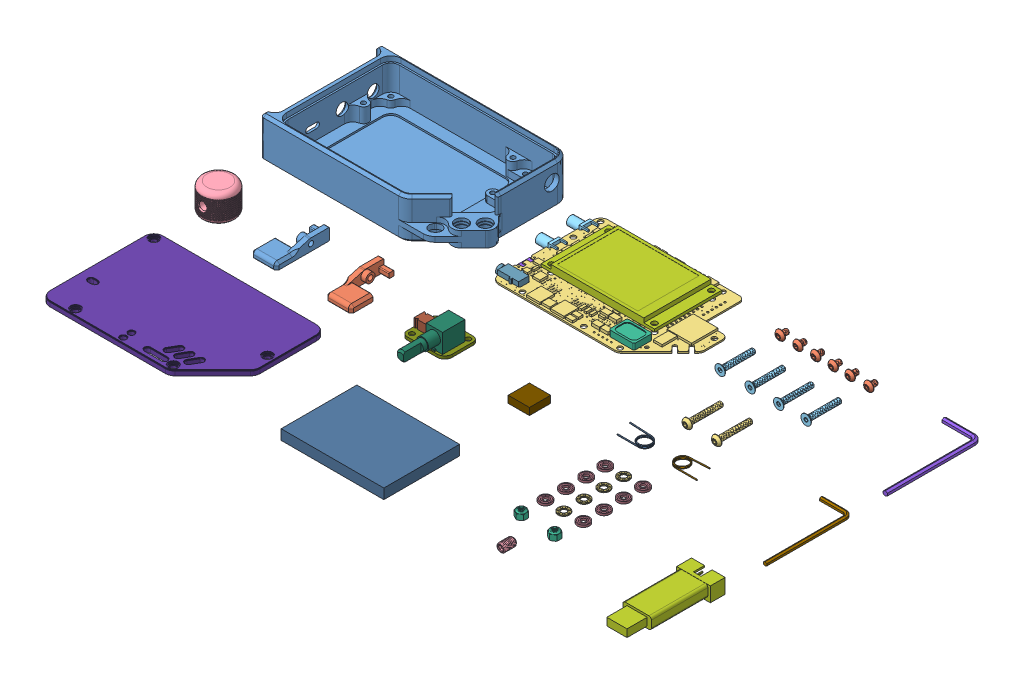
SolidWorks assembly PSDR Parts, configuration Default. Lengths in mm.
Overall size (359.88 28.12 210.13).
49 component instances, 28 part files, 92 mates.
Components (placement in the parent):
- BottomHalf2-1: BottomHalf2 [Default] at (9 12.38 68.5) x (1 0 0) z (0 1 0) size (118.23 72 24.11)
- 92095A471_18-8 SS BUTTON-HEAD SOCKET CAP SCREW-1: 92095A471_18-8 SS BUTTON-HEAD SOCKET CAP SCREW [92095A471] at (297.198 0 9.1982) x (-0.787462 -0.616364 0) z (0 0 1) size (5.7 5.7 5.93)
- 92095A185_18-8 SS BUTTON-HEAD SOCKET CAP SCREW-1: 92095A185_18-8 SS BUTTON-HEAD SOCKET CAP SCREW [92095A185] at (279.901 0 82.2808) x (0.394049 -0.919089 0) z (0 0 1) size (5.7 5.7 22.02)
- 92095A471_18-8 SS BUTTON-HEAD SOCKET CAP SCREW-2: 92095A471_18-8 SS BUTTON-HEAD SOCKET CAP SCREW [92095A471] at (244.5337 0 9.1982) x (0.999368 0.035541 0) z (0 0 1) size (5.7 5.7 5.93)
- 92029A208_TYPE 316 STAINLESS STEEL CUP POINT SET SCREW-1: 92029A208_TYPE 316 STAINLESS STEEL CUP POINT SET SCREW [92029A208] at (271.0951 0 196.8779) x (0.086276 0.996271 0) z (0 0 1) size (5.17 5.13 8.8)
- 93395A213_TYPE 316 SS FLAT-HEAD SOCKET CAP SCREW-1: 93395A213_TYPE 316 SS FLAT-HEAD SOCKET CAP SCREW [93395A213] at (244.6789 0 43.7019) x (-0.136325 -0.990664 0) z (0 0 1) size (6 6 20.36)
- 94205A220_TYPE 316 STAINLESS STEEL NYLON-INSERT LOCKNUT-1: 94205A220_TYPE 316 STAINLESS STEEL NYLON-INSERT LOCKNUT [94205A220] at (261.1628 0 178.1232) size (5.5 4.1 6.35)
- 2.2in_LCD_Module-1: 2.2in_LCD_Module [Default] at (178.3977 6.3051 29.9486) x (-1 0 0) z (0 0 -1) size (67.3 4.15 40)
- 2.5mm_Allen_Wrench-1: 2.5mm_Allen_Wrench [Default] at (357.3787 0.7217 59.475) x (0 0 1) z (-1 0 0) size (56.47 2.89 21.55)
- 2mm_Allen_Wrench-1: 2mm_Allen_Wrench [Default] at (357.8787 0.5774 131.1017) x (0 0 1) z (-1 0 0) size (51.21 2.31 17.88)
- 604561 Battery-1: 604561 Battery [Default] at (180.9722 0 187.6347) size (61 6 45)
- Battery Connector-1: Battery Connector [Default] at (139.5256 1.68 111.229) x (0 0 -1) z (1 0 0) size (6 8.6 10)
- Bearing_Inside-1: Bearing_Inside [Default] at (271.1658 0.3 162.9376) x (-0.834175 0 -0.5515) z (0.5515 0 -0.834175) size (6.7 1.25 6.7)
- Bearing_Outside-1: Bearing_Outside [Default] at (282.6637 0 150.5673) size (7 1.25 7)
- Earphone_Jack-1: Earphone_Jack [Default] at (133.0998 6.1 61.0044) x (1 0 0) z (0 0 -1) size (14.3 5.7 8.4)
- Encoder-1: Encoder [Default] at (155.9304 1.68 106.4098) x (0 0 1) z (-1 0 0) size (33.3 11.35 9.7)
- EncoderBoard-1: EncoderBoard [Default] at (93.5977 4.7 21.1162) x (0 0 1) z (0 1 0) size (20 25.5 1.68)
- Face Cover4-1: Face Cover4 [Default] at (8.7 -8.62 208.9347) x (1 0 0) z (0 1 0) size (102.4 67.4 3)
- Foam_Square-1: Foam_Square [Default] at (205.1722 0 117.3729) size (12.6 4.2 12.6)
- paddle-1: paddle [Default] at (56.1722 4 104.0749) x (0 0 1) z (0 1 0) size (31.7 15.5 7)
- paddle_Mirrored-1: paddle_Mirrored [Default] at (97.4502 4 104.0749) x (0 0 1) z (0 -1 0) size (31.7 15.5 7)
- PSDR26PCB-1: PSDR26PCB [Default] at (133.0977 2.5 67.9986) x (1 0 0) z (0 1 0) size (100 65 5.1)
- Slotted_Knob2-1: Slotted_Knob2 [Default] at (14.2624 0 111.1139) size (20.37 16 20.31)
- SMA_Connector-1: SMA_Connector [Default] at (135.0535 2.125 31.5236) x (1 0 0) z (0 0 -1) size (13.33 6.35 6.35)
- Speaker-1: Speaker [Default] at (205.0112 3.3992 57.0766) size (15 3.5 11)
- ST-Link-1: ST-Link [Default] at (349.8787 3.5 210.1347) size (20 8.7 54.3)
- USB_Connector-1: USB_Connector [Default] at (133.9105 2.5 49.0064) x (0 0 -1) z (-1 0 0) size (8.2 3.33 4.94)
- SMA_Connector-2: SMA_Connector [Default] at (135.0535 2.125 13.0361) x (1 0 0) z (0 0 -1) size (13.33 6.35 6.35)
- LeeSpring-LTML060L08S-1: LeeSpring-LTML060L08S [Default] at (282.1263 0.3047 103.5123) x (0.999674 0.025542 0) z (0 0 1) size (17.33 2.81 8.24)
- LeeSpring-LTMR060L08S-1: LeeSpring-LTMR060L08S [Default] at (260.0829 0.3047 103.7248) x (0.999674 -0.025542 0) z (0 0 1) size (17.33 2.81 8.24)
- 92095A471_18-8 SS BUTTON-HEAD SOCKET CAP SCREW-3: 92095A471_18-8 SS BUTTON-HEAD SOCKET CAP SCREW [92095A471] at (276.0216 0 9.1982) size (5.7 5.7 5.93)
- 92095A471_18-8 SS BUTTON-HEAD SOCKET CAP SCREW-4: 92095A471_18-8 SS BUTTON-HEAD SOCKET CAP SCREW [92095A471] at (255.0912 0 9.1982) x (0.635691 -0.771943 0) z (0 0 1) size (5.7 5.7 5.93)
- 92095A471_18-8 SS BUTTON-HEAD SOCKET CAP SCREW-5: 92095A471_18-8 SS BUTTON-HEAD SOCKET CAP SCREW [92095A471] at (265.6078 0 9.1982) x (0.559738 -0.82867 0) z (0 0 1) size (5.7 5.7 5.93)
- 92095A471_18-8 SS BUTTON-HEAD SOCKET CAP SCREW-6: 92095A471_18-8 SS BUTTON-HEAD SOCKET CAP SCREW [92095A471] at (286.049 0 9.1982) x (0.195213 -0.980761 0) z (0 0 1) size (5.7 5.7 5.93)
- 92095A185_18-8 SS BUTTON-HEAD SOCKET CAP SCREW-2: 92095A185_18-8 SS BUTTON-HEAD SOCKET CAP SCREW [92095A185] at (262.4328 0 82.2808) x (-0.514481 -0.857502 0) z (0 0 1) size (5.7 5.7 22.02)
- 93395A213_TYPE 316 SS FLAT-HEAD SOCKET CAP SCREW-2: 93395A213_TYPE 316 SS FLAT-HEAD SOCKET CAP SCREW [93395A213] at (295.7336 0 43.7019) x (0.996038 -0.088927 0) z (0 0 1) size (6 6 20.36)
- 93395A213_TYPE 316 SS FLAT-HEAD SOCKET CAP SCREW-3: 93395A213_TYPE 316 SS FLAT-HEAD SOCKET CAP SCREW [93395A213] at (279.4667 0 43.7019) x (0.03496 -0.999389 0) z (0 0 1) size (6 6 20.36)
- 93395A213_TYPE 316 SS FLAT-HEAD SOCKET CAP SCREW-4: 93395A213_TYPE 316 SS FLAT-HEAD SOCKET CAP SCREW [93395A213] at (262.5097 0 43.7019) x (-0.948141 0.317851 0) z (0 0 1) size (6 6 20.36)
- 94205A220_TYPE 316 STAINLESS STEEL NYLON-INSERT LOCKNUT-2: 94205A220_TYPE 316 STAINLESS STEEL NYLON-INSERT LOCKNUT [94205A220] at (281.6385 0 178.7696) size (5.5 4.1 6.35)
- Bearing_Inside-2: Bearing_Inside [Default] at (270.8814 0.3 138.8534) x (-0.998356 0 0.05732) z (-0.05732 0 -0.998356) size (6.7 1.25 6.7)
- Bearing_Inside-3: Bearing_Inside [Default] at (271.0453 0.3 127.2837) x (-0.872654 0 -0.488339) z (0.488339 0 -0.872654) size (6.7 1.25 6.7)
- Bearing_Inside-4: Bearing_Inside [Default] at (270.9927 0.3 150.7231) x (-0.987255 0 -0.159144) z (0.159144 0 -0.987255) size (6.7 1.25 6.7)
- Bearing_Outside-2: Bearing_Outside [Default] at (260.6105 0 127.7441) size (7 1.25 7)
- Bearing_Outside-3: Bearing_Outside [Default] at (260.5356 0 139.0803) size (7 1.25 7)
- Bearing_Outside-4: Bearing_Outside [Default] at (260.4639 0 150.9591) size (7 1.25 7)
- Bearing_Outside-5: Bearing_Outside [Default] at (260.2353 0 162.901) x (0.37361 0 -0.927586) z (0.927586 0 0.37361) size (7 1.25 7)
- Bearing_Outside-6: Bearing_Outside [Default] at (282.4564 0 138.6951) size (7 1.25 7)
- Bearing_Outside-7: Bearing_Outside [Default] at (282.4694 0 127.2054) x (-0.296931 0 0.954899) z (-0.954899 0 -0.296931) size (7 1.25 7)
- Bearing_Outside-8: Bearing_Outside [Default] at (282.5849 0 162.7194) size (7 1.25 7)
Mates (geometry in assembly coordinates):
- Coincident1: coincident anti-aligned: plane of BottomHalf2-1 through (82.136 0 64) normal (0 -1 0); plane of assembly through (0 0 0) normal (0 1 0)
- Coincident2: coincident anti-aligned: plane of BottomHalf2-1 through (0 -13.6924 72) normal (-1 0 0); plane of assembly through (0 0 0) normal (1 0 0)
- Coincident3: coincident anti-aligned: plane of BottomHalf2-1 through (9 -127.969 0) normal (0 0 -1); plane of assembly through (0 0 0) normal (0 0 1)
- Coincident4: coincident aligned: plane of BottomHalf2-1 through (82.136 0 64) normal (0 -1 0); plane of paddle_Mirrored-1 through (91.4502 0 104.0749) normal (0 -1 0)
- Coincident5: coincident aligned: plane of BottomHalf2-1 through (82.136 0 64) normal (0 -1 0); plane of paddle-1 through (62.1722 0 104.0749) normal (0 -1 0)
- Parallel1: parallel aligned: plane of BottomHalf2-1 through (5.5 -127.969 68.5) normal (-1 0 0); plane of paddle_Mirrored-1 through (91.4502 4 104.0749) normal (-1 0 0)
- Parallel2: parallel anti-aligned: plane of paddle-1 through (62.1722 4 104.0749) normal (1 0 0); plane of paddle_Mirrored-1 through (91.4502 4 104.0749) normal (-1 0 0)
- Coincident7: coincident aligned: plane of paddle-1 through (62.1722 4 124.7234) normal (0 0 1); plane of paddle_Mirrored-1 through (91.4502 4 124.7234) normal (0 0 1)
- Coincident8: coincident aligned: plane of BottomHalf2-1 through (82.136 0 64) normal (0 -1 0); plane of Slotted_Knob2-1 through (14.2624 0 111.1139) normal (0 -1 0)
- Coincident9: coincident aligned: plane of BottomHalf2-1 through (82.136 0 64) normal (0 -1 0); plane of Face Cover4-1 through (13.2 0 204.4347) normal (0 -1 0)
- Coincident10: coincident anti-aligned: plane of BottomHalf2-1 through (7.5 24 64) normal (1 0 0); plane of Face Cover4-1 through (7.5 3 204.4347) normal (-1 0 0)
- Coincident11: coincident anti-aligned: plane of PSDR26PCB-1 through (134.0515 3.3992 10.3266) normal (0 1 0); plane of Speaker-1 through (205.0112 3.3992 57.0766) normal (0 -1 0)
- Coincident12: coincident: axis of PSDR26PCB-1 through (214.6317 3.3992 57.0766) axis (0 -1 0); plane of Speaker-1 through (205.0112 3.3992 57.0766) normal (0 0 1)
- Lock1: lock: unknown of ?; unknown of ?
- Coincident14: coincident anti-aligned: plane of PSDR26PCB-1 through (134.0515 2.5 10.3266) normal (0 -1 0); plane of USB_Connector-1 through (151.6865 2.5 44.9064) normal (0 1 0)
- Coincident15: coincident anti-aligned: plane of PSDR26PCB-1 through (133.9105 3.3992 47.704) normal (-1 0 0); plane of USB_Connector-1 through (133.9105 2.5 49.0064) normal (1 0 0)
- Lock2: lock: unknown of ?; unknown of ?
- Coincident17: coincident anti-aligned: plane of SMA_Connector-1 through (135.0535 2.125 31.5236) normal (1 0 0); plane of PSDR26PCB-1 through (135.0535 3.3992 28.8318) normal (-1 0 0)
- Coincident18: coincident anti-aligned: plane of PSDR26PCB-1 through (135.0535 3.3992 10.3406) normal (-1 0 0); plane of SMA_Connector-2 through (135.0535 2.125 13.0361) normal (1 0 0)
- Coincident19: coincident anti-aligned: plane of PSDR26PCB-1 through (134.0515 2.5 10.3266) normal (0 -1 0); plane of SMA_Connector-1 through (135.0535 2.5 33.8886) normal (0 1 0)
- Coincident20: coincident anti-aligned: plane of PSDR26PCB-1 through (134.0515 2.5 10.3266) normal (0 -1 0); plane of SMA_Connector-2 through (135.0535 2.5 15.4011) normal (0 1 0)
- Lock3: lock: unknown of ?; unknown of ?
- Lock4: lock: unknown of ?; unknown of ?
- Coincident21: coincident anti-aligned: plane of Earphone_Jack-1 through (133.0998 2.5 61.0044) normal (0 1 0); plane of PSDR26PCB-1 through (134.0515 2.5 10.3266) normal (0 -1 0)
- Lock5: lock: unknown of ?; unknown of ?
- Concentric1: concentric aligned: cylinder of 2.2in_LCD_Module-1 through (209.0977 7.9551 47.0486) axis (0 -1 0) radius 1.65; cylinder of PSDR26PCB-1 through (209.0977 3.3992 47.0486) axis (0 -1 0) radius 1.6
- Parallel3: parallel aligned: plane of 2.2in_LCD_Module-1 through (212.0477 7.9551 9.9486) normal (0 0 -1); plane of PSDR26PCB-1 through (215.5969 3.3992 3) normal (0 0 -1)
- Distance1: distance = 4.5559 mm aligned: plane of 2.2in_LCD_Module-1 through (178.3977 7.9551 29.9486) normal (0 1 0); plane of PSDR26PCB-1 through (134.0515 3.3992 10.3266) normal (0 1 0)
- Coincident24: coincident aligned: plane of BottomHalf2-1 through (82.136 0 64) normal (0 -1 0); plane of PSDR26PCB-1 through (133.0977 0 67.9986) normal (0 -1 0)
- Coincident26: coincident aligned: plane of BottomHalf2-1 through (82.136 0 64) normal (0 -1 0); plane of EncoderBoard-1 through (154.0977 0 116.6162) normal (0 -1 0)
- Parallel4: parallel aligned: plane of BottomHalf2-1 through (9 -127.969 0) normal (0 0 -1); plane of EncoderBoard-1 through (136.0977 1.68 101.1162) normal (0 0 -1)
- Coincident27: coincident aligned: plane of BottomHalf2-1 through (82.136 0 64) normal (0 -1 0); plane of 604561 Battery-1 through (180.9722 0 187.6347) normal (0 -1 0)
- Coincident28: coincident anti-aligned: plane of Battery Connector-1 through (139.5256 1.68 111.229) normal (0 -1 0); plane of EncoderBoard-1 through (154.0977 1.68 116.6162) normal (0 1 0)
- Parallel5: parallel aligned: plane of Battery Connector-1 through (143.5256 6.78 114.229) normal (0 0 1); plane of EncoderBoard-1 through (136.0977 1.68 121.1162) normal (0 0 1)
- Lock6: lock: unknown of ?; unknown of ?
- Coincident30: coincident anti-aligned: plane of Encoder-1 through (146.2304 1.68 106.4098) normal (0 -1 0); plane of EncoderBoard-1 through (154.0977 1.68 116.6162) normal (0 1 0)
- Parallel6: parallel anti-aligned: plane of Encoder-1 through (146.2304 1.68 106.4098) normal (-1 0 0); plane of EncoderBoard-1 through (158.5977 1.68 116.6162) normal (1 0 0)
- Lock8: lock: unknown of ?; unknown of ?
- Coincident33: coincident aligned: plane of BottomHalf2-1 through (82.136 0 64) normal (0 -1 0); plane of Foam_Square-1 through (205.1722 0 117.3729) normal (0 -1 0)
- Coincident34: coincident aligned: plane of 93395A213_TYPE 316 SS FLAT-HEAD SOCKET CAP SCREW-3 through (277.9677 -0.0524 43.7019) normal (0 0 1); plane of 93395A213_TYPE 316 SS FLAT-HEAD SOCKET CAP SCREW-4 through (262.9865 1.4222 43.7019) normal (0 0 1)
- Coincident35: coincident aligned: plane of 93395A213_TYPE 316 SS FLAT-HEAD SOCKET CAP SCREW-2 through (295.6002 -1.4941 43.7019) normal (0 0 1); plane of 93395A213_TYPE 316 SS FLAT-HEAD SOCKET CAP SCREW-3 through (277.9677 -0.0524 43.7019) normal (0 0 1)
- Coincident36: coincident aligned: plane of 93395A213_TYPE 316 SS FLAT-HEAD SOCKET CAP SCREW-1 through (243.1929 0.2045 43.7019) normal (0 0 1); plane of 93395A213_TYPE 316 SS FLAT-HEAD SOCKET CAP SCREW-2 through (295.6002 -1.4941 43.7019) normal (0 0 1)
- Coincident37: coincident: plane of BottomHalf2-1 through (82.136 0 64) normal (0 -1 0); axis of 93395A213_TYPE 316 SS FLAT-HEAD SOCKET CAP SCREW-4 through (262.5097 0 42.0019) axis (0 0 -1)
- Coincident38: coincident: plane of BottomHalf2-1 through (82.136 0 64) normal (0 -1 0); axis of 93395A213_TYPE 316 SS FLAT-HEAD SOCKET CAP SCREW-3 through (279.4667 0 42.0019) axis (0 0 -1)
- Coincident39: coincident: plane of BottomHalf2-1 through (82.136 0 64) normal (0 -1 0); axis of 93395A213_TYPE 316 SS FLAT-HEAD SOCKET CAP SCREW-2 through (295.7336 0 42.0019) axis (0 0 -1)
- Coincident40: coincident: plane of BottomHalf2-1 through (82.136 0 64) normal (0 -1 0); axis of 93395A213_TYPE 316 SS FLAT-HEAD SOCKET CAP SCREW-1 through (244.6789 0 42.0019) axis (0 0 -1)
- Coincident41: coincident: plane of BottomHalf2-1 through (82.136 0 64) normal (0 -1 0); axis of 92095A185_18-8 SS BUTTON-HEAD SOCKET CAP SCREW-2 through (262.4328 0 80.6308) axis (0 0 -1)
- Coincident42: coincident: plane of BottomHalf2-1 through (82.136 0 64) normal (0 -1 0); axis of 92095A185_18-8 SS BUTTON-HEAD SOCKET CAP SCREW-1 through (279.901 0 80.6308) axis (0 0 -1)
- Coincident43: coincident: plane of BottomHalf2-1 through (82.136 0 64) normal (0 -1 0); axis of 92095A471_18-8 SS BUTTON-HEAD SOCKET CAP SCREW-1 through (297.198 0 7.5482) axis (0 0 -1)
- Coincident44: coincident: plane of BottomHalf2-1 through (82.136 0 64) normal (0 -1 0); axis of 92095A471_18-8 SS BUTTON-HEAD SOCKET CAP SCREW-6 through (286.049 0 7.5482) axis (0 0 -1)
- Coincident45: coincident: plane of BottomHalf2-1 through (82.136 0 64) normal (0 -1 0); axis of 92095A471_18-8 SS BUTTON-HEAD SOCKET CAP SCREW-3 through (276.0216 0 7.5482) axis (0 0 -1)
- Coincident46: coincident: plane of BottomHalf2-1 through (82.136 0 64) normal (0 -1 0); axis of 92095A471_18-8 SS BUTTON-HEAD SOCKET CAP SCREW-5 through (265.6078 0 7.5482) axis (0 0 -1)
- Coincident47: coincident: plane of BottomHalf2-1 through (82.136 0 64) normal (0 -1 0); axis of 92095A471_18-8 SS BUTTON-HEAD SOCKET CAP SCREW-4 through (255.0912 0 7.5482) axis (0 0 -1)
- Coincident48: coincident: plane of BottomHalf2-1 through (82.136 0 64) normal (0 -1 0); axis of 92095A471_18-8 SS BUTTON-HEAD SOCKET CAP SCREW-2 through (244.5337 0 7.5482) axis (0 0 -1)
- Coincident49: coincident: plane of BottomHalf2-1 through (82.136 0 64) normal (0 -1 0); axis of 92029A208_TYPE 316 STAINLESS STEEL CUP POINT SET SCREW-1 through (271.0951 0 193.5964) axis (0 0 1)
- Coincident50: coincident aligned: plane of BottomHalf2-1 through (82.136 0 64) normal (0 -1 0); plane of 94205A220_TYPE 316 STAINLESS STEEL NYLON-INSERT LOCKNUT-2 through (278.8885 0 174.0064) normal (0 -1 0)
- Coincident51: coincident aligned: plane of BottomHalf2-1 through (82.136 0 64) normal (0 -1 0); plane of 94205A220_TYPE 316 STAINLESS STEEL NYLON-INSERT LOCKNUT-1 through (258.4128 0 173.3601) normal (0 -1 0)
- Coincident52: coincident aligned: plane of BottomHalf2-1 through (82.136 0 64) normal (0 -1 0); plane of ST-Link-1 through (341.3787 0 164.6347) normal (0 -1 0)
- Coincident53: coincident: plane of BottomHalf2-1 through (82.136 0 64) normal (0 -1 0); line of 2.5mm_Allen_Wrench-1 through (358.6287 0 7.5) axis (0 0 1)
- Coincident54: coincident: plane of BottomHalf2-1 through (82.136 0 64) normal (0 -1 0); line of 2mm_Allen_Wrench-1 through (358.8787 0 83.8892) axis (0 0 1)
- Coincident55: coincident: plane of BottomHalf2-1 through (82.136 0 64) normal (0 -1 0); line of 2.5mm_Allen_Wrench-1 through (355.3787 0 4.25) axis (-1 0 0)
- Coincident56: coincident: plane of BottomHalf2-1 through (82.136 0 64) normal (0 -1 0); line of 2mm_Allen_Wrench-1 through (355.8787 0 80.8892) axis (-1 0 0)
- Coincident57: coincident aligned: plane of BottomHalf2-1 through (82.136 0 64) normal (0 -1 0); plane of Bearing_Outside-2 through (260.6105 0 127.7441) normal (0 -1 0)
- Coincident58: coincident aligned: plane of BottomHalf2-1 through (82.136 0 64) normal (0 -1 0); plane of Bearing_Outside-1 through (282.6637 0 150.5673) normal (0 -1 0)
- Coincident59: coincident aligned: plane of BottomHalf2-1 through (82.136 0 64) normal (0 -1 0); plane of Bearing_Outside-8 through (282.5849 0 162.7194) normal (0 -1 0)
- Coincident60: coincident anti-aligned: plane of BottomHalf2-1 through (82.136 0 64) normal (0 -1 0); circle of Bearing_Outside-7
- Coincident61: coincident aligned: plane of BottomHalf2-1 through (82.136 0 64) normal (0 -1 0); plane of Bearing_Outside-3 through (260.5356 0 139.0803) normal (0 -1 0)
- Coincident62: coincident aligned: plane of BottomHalf2-1 through (82.136 0 64) normal (0 -1 0); plane of Bearing_Outside-6 through (282.4564 0 138.6951) normal (0 -1 0)
- Coincident63: coincident anti-aligned: plane of BottomHalf2-1 through (82.136 0 64) normal (0 -1 0); circle of Bearing_Outside-5
- Coincident64: coincident aligned: plane of BottomHalf2-1 through (82.136 0 64) normal (0 -1 0); plane of Bearing_Outside-4 through (260.4639 0 150.9591) normal (0 -1 0)
- Coincident65: coincident anti-aligned: plane of BottomHalf2-1 through (82.136 0 64) normal (0 -1 0); circle of Bearing_Inside-2
- Coincident66: coincident anti-aligned: plane of BottomHalf2-1 through (82.136 0 64) normal (0 -1 0); circle of Bearing_Inside-1
- Coincident67: coincident anti-aligned: plane of BottomHalf2-1 through (82.136 0 64) normal (0 -1 0); circle of Bearing_Inside-3
- Coincident68: coincident anti-aligned: plane of BottomHalf2-1 through (82.136 0 64) normal (0 -1 0); circle of Bearing_Inside-4
- Tangent3: tangent: plane of BottomHalf2-1 through (82.136 0 64) normal (0 -1 0); face of LeeSpring-LTML060L08S-1
- Tangent4: tangent: plane of BottomHalf2-1 through (82.136 0 64) normal (0 -1 0); face of LeeSpring-LTMR060L08S-1
- Coincident69: coincident aligned: plane of 92095A185_18-8 SS BUTTON-HEAD SOCKET CAP SCREW-1 through (277.2816 -1.123 80.6308) normal (0 0 -1); plane of 92095A185_18-8 SS BUTTON-HEAD SOCKET CAP SCREW-2 through (259.989 1.4663 80.6308) normal (0 0 -1)
- Coincident70: coincident aligned: plane of 92095A471_18-8 SS BUTTON-HEAD SOCKET CAP SCREW-1 through (295.4414 2.2443 7.5482) normal (0 0 -1); plane of 92095A471_18-8 SS BUTTON-HEAD SOCKET CAP SCREW-2 through (244.6349 -2.8482 7.5482) normal (0 0 -1)
- Coincident71: coincident aligned: plane of 92095A471_18-8 SS BUTTON-HEAD SOCKET CAP SCREW-1 through (295.4414 2.2443 7.5482) normal (0 0 -1); plane of 92095A471_18-8 SS BUTTON-HEAD SOCKET CAP SCREW-4 through (252.8911 -1.8117 7.5482) normal (0 0 -1)
- Coincident72: coincident aligned: plane of 92095A471_18-8 SS BUTTON-HEAD SOCKET CAP SCREW-4 through (252.8911 -1.8117 7.5482) normal (0 0 -1); plane of 92095A471_18-8 SS BUTTON-HEAD SOCKET CAP SCREW-5 through (263.2461 -1.5953 7.5482) normal (0 0 -1)
- Coincident73: coincident aligned: plane of 92095A471_18-8 SS BUTTON-HEAD SOCKET CAP SCREW-3 through (276.0216 -2.85 7.5482) normal (0 0 -1); plane of 92095A471_18-8 SS BUTTON-HEAD SOCKET CAP SCREW-5 through (263.2461 -1.5953 7.5482) normal (0 0 -1)
- Coincident74: coincident aligned: plane of 92095A471_18-8 SS BUTTON-HEAD SOCKET CAP SCREW-3 through (276.0216 -2.85 7.5482) normal (0 0 -1); plane of 92095A471_18-8 SS BUTTON-HEAD SOCKET CAP SCREW-6 through (283.2538 -0.5564 7.5482) normal (0 0 -1)
- Parallel7: parallel aligned: plane of BottomHalf2-1 through (5.5 -127.969 68.5) normal (-1 0 0); plane of 2.5mm_Allen_Wrench-1 through (357.3787 2.1651 7.5) normal (-1 0 0)
- Parallel8: parallel aligned: plane of BottomHalf2-1 through (5.5 -127.969 68.5) normal (-1 0 0); plane of 2mm_Allen_Wrench-1 through (357.8787 1.7321 83.8892) normal (-1 0 0)
- Coincident75: coincident anti-aligned: plane of BottomHalf2-1 through (9 -127.969 3) normal (0 0 1); plane of PSDR26PCB-1 through (215.5969 3.3992 3) normal (0 0 -1)
- Coincident76: coincident aligned: plane of EncoderBoard-1 through (133.0977 1.68 118.1162) normal (-1 0 0); plane of PSDR26PCB-1 through (133.0977 3.3992 54.0032) normal (-1 0 0)
- Coincident78: coincident aligned: plane of 604561 Battery-1 through (150.4722 6 210.1347) normal (0 0 1); plane of Face Cover4-1 through (81.836 3 210.1347) normal (0 0 1)
- Coincident79: coincident aligned: plane of 2.5mm_Allen_Wrench-1 through (359.8787 0.7217 7.5) normal (1 0 0); plane of 2mm_Allen_Wrench-1 through (359.8787 0.5774 83.8892) normal (1 0 0)
- Coincident80: coincident aligned: plane of 2mm_Allen_Wrench-1 through (359.8787 0.5774 83.8892) normal (1 0 0); plane of ST-Link-1 through (359.8787 7.1 155.8347) normal (1 0 0)
- Coincident81: coincident aligned: plane of 604561 Battery-1 through (150.4722 6 210.1347) normal (0 0 1); plane of ST-Link-1 through (349.8787 3.5 210.1347) normal (0 0 1)
- Coincident82: coincident aligned: plane of 2.5mm_Allen_Wrench-1 through (355.3787 0.7217 3) normal (0 0 -1); plane of PSDR26PCB-1 through (215.5969 3.3992 3) normal (0 0 -1)
- Coincident83: coincident aligned: plane of 604561 Battery-1 through (211.4722 6 210.1347) normal (1 0 0); plane of Foam_Square-1 through (211.4722 4.2 123.6729) normal (1 0 0)
